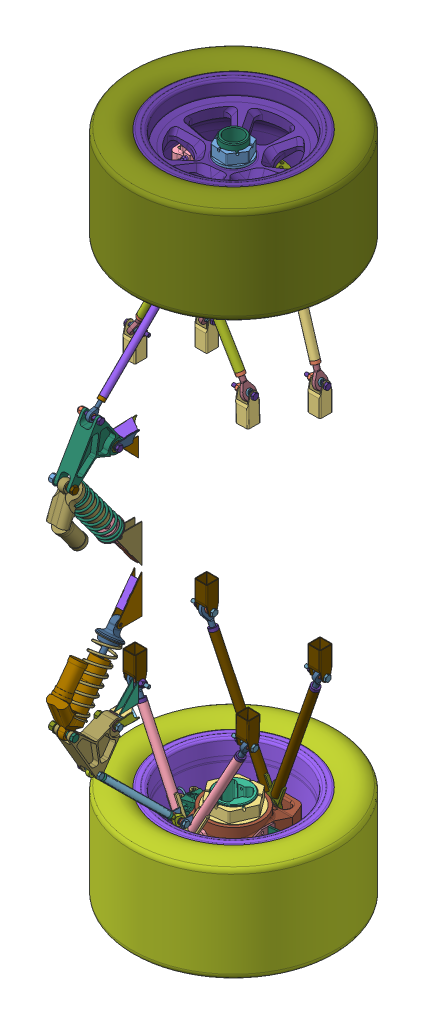
SolidWorks assembly UN-A1001-AA-Rear Unsprung Assembly, configuration Default. Lengths in mm. (continued)
Components (placement in the parent): (continued)
- MirrorWT-A0100-XG-Corner Assembly-2: MirrorWT-A0100-XG-Corner Assembly [Default] x (1 0 0) z (0 0 -1) size (411.48 213.6 411.53) (continued)
  - MirrorBR-A0000-AB-Rear Brake Assembly-1: MirrorBR-A0000-AB-Rear Brake Assembly [Default] at (-793.1174 596.9879 -198.9034) x (-0.602494 -0.000202 0.798123) z (0.798123 -0.000152 0.602494) size (251.55 172.72 251.55) (continued)
    - MirrorBR-20603-BA-Floating Bobbins-4: MirrorBR-20603-BA-Floating Bobbins [Default] at (-39.8696 25.9874 23.0188) x (-1 0 0) z (0 0 -1) size (15.88 8.92 15.88)
    - MirrorBR-20603-BA-Floating Bobbins-5: MirrorBR-20603-BA-Floating Bobbins [Default] at (0 25.9874 46.0375) x (-0.5 0 0.866025) z (-0.866025 0 -0.5) size (15.88 8.92 15.88)
    - MirrorBR-20603-BA-Floating Bobbins-6: MirrorBR-20603-BA-Floating Bobbins [Default] at (39.8696 25.9874 23.0188) x (0.5 0 0.866025) z (-0.866025 0 0.5) size (15.88 8.92 15.88)
    - MirrorWT-20104-AB-Rear Sensor Ring-1: MirrorWT-20104-AB-Rear Sensor Ring [Default] at (0 30.099 0) x (-0.882948 0 -0.469472) z (0 1 0) size (137 137 1.59)
    - Mirror91590A121_External Retaining Ring-1: Mirror91590A121_External Retaining Ring [91590A121] at (-39.8696 29.2354 -23.0188) x (0 1 0) z (0.857167 0 0.515038) size (0.64 14.63 13.25)
    - Mirror91590A121_External Retaining Ring-2: Mirror91590A121_External Retaining Ring [91590A121] at (-39.8696 29.2354 23.0188) x (0 1 0) z (0.87462 0 -0.48481) size (0.64 14.63 13.25)
    - Mirror91590A121_External Retaining Ring-3: Mirror91590A121_External Retaining Ring [91590A121] at (0 29.2354 46.0375) x (0 1 0) z (0.017452 0 -0.999848) size (0.64 14.63 13.25)
    - Mirror91590A121_External Retaining Ring-4: Mirror91590A121_External Retaining Ring [91590A121] at (39.8696 29.2354 23.0188) x (0 1 0) z (-0.857167 0 -0.515038) size (0.64 14.63 13.25)
    - Mirror91590A121_External Retaining Ring-5: Mirror91590A121_External Retaining Ring [91590A121] at (39.8696 29.2354 -23.0188) x (0 1 0) z (-0.87462 0 0.48481) size (0.64 14.63 13.25)
    - Mirror91590A121_External Retaining Ring-6: Mirror91590A121_External Retaining Ring [91590A121] at (0 29.2354 -46.0375) x (0 1 0) z (-0.017452 0 0.999848) size (0.64 14.63 13.25)
    - Mirror97447A110_Aluminum Blind Rivets with Aluminum Mandrel-1: Mirror97447A110_Aluminum Blind Rivets with Aluminum Mandrel [97447A110] at (9.6137 30.099 -51.8707) x (-0.302097 0 0.953277) z (0 -1 0) size (5.03 5.03 11.56)
    - Mirror97447A110_Aluminum Blind Rivets with Aluminum Mandrel-2: Mirror97447A110_Aluminum Blind Rivets with Aluminum Mandrel [97447A110] at (-40.1145 30.099 -34.261) x (0.674514 0 0.738262) z (0 -1 0) size (5.03 5.03 11.56)
    - Mirror97447A110_Aluminum Blind Rivets with Aluminum Mandrel-3: Mirror97447A110_Aluminum Blind Rivets with Aluminum Mandrel [97447A110] at (-49.7282 30.099 17.6097) x (0.976611 0 -0.215015) z (0 -1 0) size (5.03 5.03 11.56)
    - Mirror97447A110_Aluminum Blind Rivets with Aluminum Mandrel-4: Mirror97447A110_Aluminum Blind Rivets with Aluminum Mandrel [97447A110] at (-9.6137 30.099 51.8707) x (0.302097 0 -0.953277) z (0 -1 0) size (5.03 5.03 11.56)
    - Mirror97447A110_Aluminum Blind Rivets with Aluminum Mandrel-5: Mirror97447A110_Aluminum Blind Rivets with Aluminum Mandrel [97447A110] at (40.1145 30.099 34.261) x (-0.674514 0 -0.738262) z (0 -1 0) size (5.03 5.03 11.56)
    - Mirror97447A110_Aluminum Blind Rivets with Aluminum Mandrel-6: Mirror97447A110_Aluminum Blind Rivets with Aluminum Mandrel [97447A110] at (49.7282 30.099 -17.6097) x (-0.976611 0 0.215015) z (0 -1 0) size (5.03 5.03 11.56)
  - MirrorFS-Jet Nut, M8x1.25 (MJET-M8X1.25)-1: MirrorFS-Jet Nut, M8x1.25 (MJET-M8X1.25) [Default] at (-816.1783 561.0546 -293.5333) x (-0.906747 0.01433 0.421432) z (0.000308 -0.9994 0.034645) size (13.6 13.6 7)
  - Mirror91290A442_Alloy Steel Socket Head Screw-2: Mirror91290A442_Alloy Steel Socket Head Screw [91290A442] at (-771.7287 556.8303 -293.7791) x (-0.549228 0.028783 0.835176) z (-0.000308 0.9994 -0.034645) size (13 13 48.09)
  - MirrorFS-Jet Nut, M8x1.25 (MJET-M8X1.25)-2: MirrorFS-Jet Nut, M8x1.25 (MJET-M8X1.25) [Default] at (-771.73 561.0547 -293.9256) x (0.139109 0.034351 0.989681) z (0.000308 -0.9994 0.034645) size (13.6 13.6 7)
  - MirrorWT-10105-AA-Drive Pin-2: MirrorWT-10105-AA-Drive Pin [Default] at (-769.0177 596.9959 -230.8283) x (0.992582 0.000031 -0.121576) z (0.121576 -0.000251 0.992582) size (12.67 23.01 11.95)
  - MirrorWT-10105-AA-Drive Pin-3: MirrorWT-10105-AA-Drive Pin [Default] at (-761.1925 596.9818 -174.8036) x (0.121576 -0.000251 0.992582) z (-0.992582 -0.000031 0.121576) size (12.67 23.01 11.95)
  - MirrorWT-10105-AA-Drive Pin-4: MirrorWT-10105-AA-Drive Pin [Default] at (-817.2172 596.9798 -166.9785) x (-0.992582 -0.000031 0.121576) z (-0.121576 0.000251 -0.992582) size (12.67 23.01 11.95)
  - MirrorWT-AA-#####-Rear Toe Backing Plate-1: MirrorWT-AA-#####-Rear Toe Backing Plate [Default] at (-737.6079 537.8924 -199.4082) x (0.999961 0.000002 -0.008824) z (0.008824 -0.000253 0.999961) size (3.17 25.4 50.8)
  - MirrorWT-AA-#####-Rear Toe Top Clevis-1: MirrorWT-AA-#####-Rear Toe Top Clevis [Default] at (-737.7085 541.0703 -210.8115) x (0.999961 0.000002 -0.008824) z (0.008824 -0.000253 0.999961) size (31.75 27.83 3.17)
  - MirrorWT-AA-#####-Rear Toe Bottom Clevis-1: MirrorWT-AA-#####-Rear Toe Bottom Clevis [Default] at (-737.4815 537.8888 -185.0832) x (0.999961 0.000002 -0.008824) z (0.008824 -0.000253 0.999961) size (31.75 27.12 3.17)
- MirrorSP-A0200-AH-Rear Axle Assembly-3: MirrorSP-A0200-AH-Rear Axle Assembly [Default] x (1 0 0) z (0 0 -1) size (274.88 563.57 484.64)
  - MirrorSP-AA-Rear Lower A-Arm^SP-A0200-AH-Rear Axle Assembly-1: MirrorSP-AA-Rear Lower A-Arm^SP-A0200-AH-Rear Axle Assembly [Default] at (0 -0.399 -0.6588) x (1 0 0) z (0 -0.002866 0.999996) size (222.76 290.57 36.42)
    - MirrorSP-Lower Apex Rear-1: MirrorSP-Lower Apex Rear [Default] at (-792.4265 549.6462 -121.5417) x (-0.932505 -0.360479 -0.022123) z (0 0.061256 -0.998122) size (54.94 63.8 9.53)
    - MirrorMirrorFS-MALE ROD END UNF-3A, 0.3125x24-0.25D (XAM-4)14-1: MirrorMirrorFS-MALE ROD END UNF-3A, 0.3125x24-0.25D (XAM-4)14 [Default] at (-906.7265 255.0788 -139.6197) x (0.932505 -0.360479 -0.022123) z (0.361157 0.930754 0.057121)
    - MirrorMirrorFS-MALE ROD END UNF-3A, 0.3125x24-0.25D (XAM-4)15-1: MirrorMirrorFS-MALE ROD END UNF-3A, 0.3125x24-0.25D (XAM-4)15 [Default] at (-678.1265 255.0788 -139.6197) x (0.932505 0.360479 0.022123) z (-0.361157 0.930754 0.057121)
    - MirrorSP-10003-AB-Threaded Insert-1: MirrorSP-10003-AB-Threaded Insert [A-Arm] at (-890.6731 296.4508 -137.0806) x (0.932505 -0.360479 -0.022123) z (0.361157 0.930754 0.057121) size (15.88 15.88 15.88)
    - MirrorSP-10003-AB-Threaded Insert-2: MirrorSP-10003-AB-Threaded Insert [A-Arm] at (-694.18 296.4508 -137.0806) x (0.932505 0.360479 0.022123) z (-0.361157 0.930754 0.057121) size (15.88 15.88 15.88)
    - MirrorSP-Rear Lower A-Arm Tube-1: MirrorSP-Rear Lower A-Arm Tube [Default] at (-838.6322 430.5677 -128.8497) x (-0.361157 -0.930754 -0.057121) z (0 0.061256 -0.998122) size (257.84 15.88 15.88)
    - MirrorSP-Rear Lower A-Arm Tube-2: MirrorSP-Rear Lower A-Arm Tube [Default] at (-746.2209 430.5677 -128.8497) x (0.361157 -0.930754 -0.057121) z (0 -0.061256 0.998122) size (257.84 15.88 15.88)
    - MirrorFS-HIGH MISALIGN SPHERICAL BEARING, 0.375-0.906D (3072-6G)2-1: MirrorFS-HIGH MISALIGN SPHERICAL BEARING, 0.375-0.906D (3072-6G)2 [Default] at (-792.4265 549.6462 -121.5417) x (-0.932505 0.360479 0.022123) z (0.361157 0.930754 0.057121) size (26.46 21.71 26.13)
      - MirrorRace^FS-HIGH MISALIGN SPHERICAL BEARING, 0.375-0.906D (3072-6G)-1: MirrorRace^FS-HIGH MISALIGN SPHERICAL BEARING, 0.375-0.906D (3072-6G) [Default] at origin size (23.01 8.76 23.01) (virtual)
      - MirrorBall^FS-HIGH MISALIGN SPHERICAL BEARING, 0.375-0.906D (3072-6G)-1: MirrorBall^FS-HIGH MISALIGN SPHERICAL BEARING, 0.375-0.906D (3072-6G) [Default] x (0.359576 -0.008176 -0.93308) z (0.932238 0.046516 0.358844) size (19.84 20.65 19.84) (virtual)
  - MirrorSP-AA-Rear Upper A-Arm^SP-A0200-AH-Rear Axle Assembly-1: MirrorSP-AA-Rear Upper A-Arm^SP-A0200-AH-Rear Axle Assembly [Default] at (-38.1 -1.9308 -1.9372) x (1 0 0) z (0 -0.00685 0.999977) size (216 215.55 29.43)
    - MirrorSP-Upper Apex Rear-1: MirrorSP-Upper Apex Rear [Default] at (-755.8405 523.8827 -293.8505) x (0.884705 -0.465567 0.023329) z (0 0.050046 0.998747) size (76.45 83.12 9.53)
    - MirrorMirrorFS-MALE ROD END UNF-3A, 0.3125x24-0.25D (XAM-4)16-1: MirrorMirrorFS-MALE ROD END UNF-3A, 0.3125x24-0.25D (XAM-4)16 [Default] at (-870.1405 307.2255 -282.9942) x (0.884705 -0.465567 0.023329) z (0.466151 0.883596 -0.044276)
    - MirrorMirrorFS-MALE ROD END UNF-3A, 0.3125x24-0.25D (XAM-4)17-1: MirrorMirrorFS-MALE ROD END UNF-3A, 0.3125x24-0.25D (XAM-4)17 [Default] at (-641.5405 307.2255 -282.9942) x (0.884705 0.465567 -0.023329) z (-0.466151 0.883596 -0.044276)
    - MirrorSP-10003-AB-Threaded Insert-1: MirrorSP-10003-AB-Threaded Insert [A-Arm] at (-849.4201 346.5014 -284.9623) x (0.884705 -0.465567 0.023329) z (0.466151 0.883596 -0.044276) size (15.88 15.88 15.88)
    - MirrorSP-10003-AB-Threaded Insert-2: MirrorSP-10003-AB-Threaded Insert [A-Arm] at (-662.261 346.5014 -284.9623) x (0.884705 0.465567 -0.023329) z (-0.466151 0.883596 -0.044276) size (15.88 15.88 15.88)
    - MirrorSP-Rear Upper A-Arm Tube-1: MirrorSP-Rear Upper A-Arm Tube [Default] at (-812.9905 415.5541 -288.4224) x (0.466151 0.883596 -0.044276) z (-0.884705 0.465567 -0.023329) size (186.28 15.88 15.88)
    - MirrorSP-Rear Upper A-Arm Tube-2: MirrorSP-Rear Upper A-Arm Tube [Default] at (-698.6905 415.5541 -288.4224) x (-0.466151 0.883596 -0.044276) z (-0.884705 -0.465567 0.023329) size (186.28 15.88 15.88)
    - MirrorFS-HIGH MISALIGN SPHERICAL BEARING, 0.375-0.906D (3072-6G)3-1: MirrorFS-HIGH MISALIGN SPHERICAL BEARING, 0.375-0.906D (3072-6G)3 [Default] at (-755.8405 523.8827 -293.8505) x (0.884705 -0.465567 0.023329) z (0.466151 0.883596 -0.044276) size (26.46 21.71 26.13)
      - MirrorRace^FS-HIGH MISALIGN SPHERICAL BEARING, 0.375-0.906D (3072-6G)-1: MirrorRace^FS-HIGH MISALIGN SPHERICAL BEARING, 0.375-0.906D (3072-6G) [Default] at origin size (23.01 8.76 23.01) (virtual)
      - MirrorBall^FS-HIGH MISALIGN SPHERICAL BEARING, 0.375-0.906D (3072-6G)-1: MirrorBall^FS-HIGH MISALIGN SPHERICAL BEARING, 0.375-0.906D (3072-6G) [Default] x (0.359576 -0.008176 -0.93308) z (0.932238 0.046516 0.358844) size (19.84 20.65 19.84) (virtual)
  - MirrorAssem8^SP-A0200-AH-Rear Axle Assembly-1: MirrorAssem8^SP-A0200-AH-Rear Axle Assembly [Default] at (-1592.9214 814.7933 -712.2762) x (-0.999891 -0.01037 -0.010464) z (-0.012143 0.982316 0.186836) size (17.98 166.51 230.13)
    - MirrorPart2^Assem8_SP-A0200-AH-Rear Axle Assembly-1: MirrorPart2^Assem8_SP-A0200-AH-Rear Axle Assembly [Default] at origin size (15.39 113.92 157.78) (virtual)
    - MirrorSP-10003-AC-Threaded Insert-1: MirrorSP-10003-AC-Threaded Insert [AM-4 Rod End Thread] at (-799.064 427.6015 -294.0449) x (-0.999891 -0.008342 -0.012143) z (0.014733 -0.566176 -0.824153) size (12.7 12.7 15.88)
    - MirrorSP-10003-AC-Threaded Insert-2: MirrorSP-10003-AC-Threaded Insert [AM-4 Rod End Thread] at (-796.6527 334.9355 -428.9338) x (-0.999891 -0.008342 -0.012143) z (-0.014733 0.566176 0.824153) size (12.7 12.7 15.88)
    - MirrorFS-MALE ROD END UNF-3A, 0.25x28-0.25D (AM-4)2-1: MirrorFS-MALE ROD END UNF-3A, 0.25x28-0.25D (AM-4)2 [Default] at (-796.0446 311.5665 -462.9507) x (0 -0.824242 0.566238) z (0.014733 -0.566176 -0.824153) size (19.32 14.06 49.44)
      - MirrorBody^FS-MALE ROD END UNF-3A, 0.25x28-0.25D (AM-4)-1: MirrorBody^FS-MALE ROD END UNF-3A, 0.25x28-0.25D (AM-4) [Default] at origin size (19.32 7.2 49.44) (virtual)
      - MirrorBall^FS-MALE ROD END UNF-3A, 0.25x28-0.25D (AM-4)-1: MirrorBall^FS-MALE ROD END UNF-3A, 0.25x28-0.25D (AM-4) [Default] x (0.09633 0.218783 -0.971007) z (0.984027 -0.167661 0.059845) size (12.7 9.53 12.7) (virtual)
    - MirrorFS-MALE ROD END UNF-3A, 0.25x28-0.25D (AM-4)3-1: MirrorFS-MALE ROD END UNF-3A, 0.25x28-0.25D (AM-4)3 [Default] at (-799.6721 450.9704 -260.028) x (0 -0.824242 0.566238) z (-0.014733 0.566176 0.824153) size (19.32 14.06 49.44)
      - MirrorBody^FS-MALE ROD END UNF-3A, 0.25x28-0.25D (AM-4)-1: MirrorBody^FS-MALE ROD END UNF-3A, 0.25x28-0.25D (AM-4) [Default] at origin size (19.32 7.2 49.44) (virtual)
      - MirrorBall^FS-MALE ROD END UNF-3A, 0.25x28-0.25D (AM-4)-1: MirrorBall^FS-MALE ROD END UNF-3A, 0.25x28-0.25D (AM-4) [Default] x (0.09633 0.218783 -0.971007) z (0.984027 -0.167661 0.059845) size (12.7 9.53 12.7) (virtual)
  - MirrorSP-A0105-AC-Ohlin TTX25 MKII, 200mm1-1: MirrorSP-A0105-AC-Ohlin TTX25 MKII, 200mm1 [Default] at (-793.9406 216.4917 -537.8809) x (-1 0 0) z (0 -0.803503 0.5953) size (48.39 85.02 197.6)
    - MirrorShock Body^SP-A0105-AC-Ohlin TTX25 MKII, 200mm-1: MirrorShock Body^SP-A0105-AC-Ohlin TTX25 MKII, 200mm [Default] at origin size (40.76 80 131.7) (virtual)
    - MirrorHead^SP-A0105-AC-Ohlin TTX25 MKII, 200mm-1: MirrorHead^SP-A0105-AC-Ohlin TTX25 MKII, 200mm [Default] at (0 0 174.6) size (46 46 119) (virtual)
    - MirrorBall^SP-A0105-AC-Ohlin TTX25 MKII, 200mm-1: MirrorBall^SP-A0105-AC-Ohlin TTX25 MKII, 200mm [Default] at (0 0 174.6) x (-0.011681 0.107343 -0.994153) z (-0.993776 -0.111394 -0.000351) size (15 15 8) (virtual)
    - MirrorBall^SP-A0105-AC-Ohlin TTX25 MKII, 200mm-2: MirrorBall^SP-A0105-AC-Ohlin TTX25 MKII, 200mm [Default] x (0.079523 -0.862756 0.499328) z (-0.965926 0.057074 0.252448) size (15 15 8) (virtual)
    - MirrorSP-#####-AB-Spring-1: MirrorSP-#####-AB-Spring [Default] at (0 0 151.1) size (48.39 49.05 127.97)
  - MirrorFS-BALL BEARING, 0.25ID-0.75OD (60355K702)-1: MirrorFS-BALL BEARING, 0.25ID-0.75OD (60355K702) [Default] at (-784.8125 243.84 -446.6415) x (0 -0.287121 -0.957894) z (1 0 0) size (19.05 19.05 7.14)
  - MirrorFS-BALL BEARING, 0.25ID-0.75OD (60355K702)-2: MirrorFS-BALL BEARING, 0.25ID-0.75OD (60355K702) [Default] at (-803.0688 243.84 -446.6415) x (0 0.287121 0.957894) z (-1 0 0) size (19.05 19.05 7.14)
  - MirrorFS-CADMIUM PLATED C3 HEX, 0.25x28-1.65-0.469 (AN4-13A)-1: MirrorFS-CADMIUM PLATED C3 HEX, 0.25x28-1.65-0.469 (AN4-13A) [Default] at (-796.8362 310.0391 -484.3789) x (-1 0 0) z (0 -0.868755 0.495242) size (46.28 12.9 11.18)
  - MirrorFS-ZINC YELLOW CHROMATE C10.9 HX, M8x1.25-40-22 (95327A569)-1: MirrorFS-ZINC YELLOW CHROMATE C10.9 HX, M8x1.25-40-22 (95327A569) [Default] at (-795.4156 216.4917 -537.8809) x (-1 0 0) z (0 0.287121 0.957894) size (45.3 15.01 13)
  - MirrorFS-NYLOC FLHX C8, M8x1.25-11.1 (92461A400)-1: MirrorFS-NYLOC FLHX C8, M8x1.25-11.1 (92461A400) [Default] at (-820.9156 216.4917 -537.8809) x (0 0.868058 0.496463) z (1 0 0) size (17.9 17.9 11.1)
  - MirrorFS-NYLOC G8 HX, 0.25x28-0.3125 (90630A145)-1: MirrorFS-NYLOC G8 HX, 0.25x28-0.3125 (90630A145) [Default] at (-809.8156 310.0391 -484.3789) x (0 0.868058 0.496463) z (0 -0.496463 0.868058) size (11.11 7.94 12.83)
  - MirrorSP-C30066-AA-A-Arm Tab Box-1: MirrorSP-C30066-AA-A-Arm Tab Box [Default] at (-680.9758 289.7175 -282.8202) x (-0.029021 0.999579 0) z (0 0 -1) size (60.32 25.4 25.4)
  - MirrorSP-C30066-AA-A-Arm Tab Box-2: MirrorSP-C30066-AA-A-Arm Tab Box [Default] at (-908.2405 289.7636 -282.8202) x (0 1 0) z (0 0 -1) size (60.32 25.4 25.4)
  - MirrorSP-C30066-AA-A-Arm Tab Box-3: MirrorSP-C30066-AA-A-Arm Tab Box [Default] at (-678.1265 237.6164 -139.5469) x (0 1 0) z (0 0 1) size (60.32 25.4 25.4)
  - MirrorSP-C30066-AA-A-Arm Tab Box-4: MirrorSP-C30066-AA-A-Arm Tab Box [Default] at (-906.7265 237.6164 -139.5469) x (0 1 0) z (0 0 1) size (60.32 25.4 25.4)
  - MirrorMirrorSP-30063-AB-Pushrod Tab-1: MirrorMirrorSP-30063-AB-Pushrod Tab [Default] at (-782.0343 483.2134 -293.6084) x (1 0 0) z (0 -0.043203 -0.999066) size (1.59 15.88 23.81)
  - MirrorMirrorSP-30063-AB-Pushrod Tab-2: MirrorMirrorSP-30063-AB-Pushrod Tab [Default] at (-805.8468 483.2134 -293.6084) x (-1 0 0) z (0 -0.043203 -0.999066) size (1.59 15.88 23.81)
  - MirrorFS-NYLOC FLHX C8, M8x1.25-11.1 (92461A400)-2: MirrorFS-NYLOC FLHX C8, M8x1.25-11.1 (92461A400) [Default] at (-820.9156 243.84 -446.6415) x (0 0 1) z (1 0 0) size (17.9 17.9 11.1)
  - MirrorFS-CADMIUM PLATED C3 HEX, 0.25x28-1.65-0.469 (AN4-13A)-2: MirrorFS-CADMIUM PLATED C3 HEX, 0.25x28-1.65-0.469 (AN4-13A) [Default] at (-796.8362 243.84 -446.6415) x (-1 0 0) z (0 -0.287121 -0.957894) size (46.28 12.9 11.18)
  - MirrorFS-CADMIUM PLATED C3 HEX, 0.25x28-1.65-0.469 (AN4-13A)-3: MirrorFS-CADMIUM PLATED C3 HEX, 0.25x28-1.65-0.469 (AN4-13A) [Default] at (-687.5506 306.9965 -282.8202) x (-0.999579 -0.029021 0) z (0 0 -1) size (46.28 12.9 11.18)
  - MirrorFS-CADMIUM PLATED C3 HEX, 0.25x28-1.65-0.469 (AN4-13A)-4: MirrorFS-CADMIUM PLATED C3 HEX, 0.25x28-1.65-0.469 (AN4-13A) [Default] at (-902.1699 307.2261 -282.8202) size (46.28 12.9 11.18)
  - MirrorFS-CADMIUM PLATED C3 HEX, 0.25x28-1.65-0.469 (AN4-13A)-5: MirrorFS-CADMIUM PLATED C3 HEX, 0.25x28-1.65-0.469 (AN4-13A) [Default] at (-912.7971 255.0789 -139.5469) x (-1 0 0) z (0 0 -1) size (46.28 12.9 11.18)
  - MirrorFS-CADMIUM PLATED C3 HEX, 0.25x28-1.65-0.469 (AN4-13A)-6: MirrorFS-CADMIUM PLATED C3 HEX, 0.25x28-1.65-0.469 (AN4-13A) [Default] at (-684.1971 255.0789 -139.5469) x (-1 0 0) z (0 0 -1) size (46.28 12.9 11.18)
  - MirrorFS-CADMIUM PLATED C3 HEX, 0.25x28-1.65-0.469 (AN4-13A)-7: MirrorFS-CADMIUM PLATED C3 HEX, 0.25x28-1.65-0.469 (AN4-13A) [Default] at (-799.2174 482.5275 -309.4686) x (-1 0 0) z (0 0.609051 0.793131) size (46.28 12.9 11.18)
  - MirrorFS-NYLOC G8 HX, 0.25x28-0.3125 (90630A145)-2: MirrorFS-NYLOC G8 HX, 0.25x28-0.3125 (90630A145) [Default] at (-807.4343 482.5275 -309.4686) x (0 -0.043203 -0.999066) z (0 0.999066 -0.043203) size (11.11 7.94 12.83)
  - MirrorFS-NYLOC G8 HX, 0.25x28-0.3125 (90630A145)-3: MirrorFS-NYLOC G8 HX, 0.25x28-0.3125 (90630A145) [Default] at (-694.1772 306.8041 -282.8202) x (-0.029021 0.999579 0) z (0 0 1) size (11.11 7.94 12.83)
  - MirrorFS-NYLOC G8 HX, 0.25x28-0.3125 (90630A145)-4: MirrorFS-NYLOC G8 HX, 0.25x28-0.3125 (90630A145) [Default] at (-895.5405 307.2261 -282.8202) x (0 1 0) z (0 0 -1) size (11.11 7.94 12.83)
  - MirrorFS-NYLOC G8 HX, 0.25x28-0.3125 (90630A145)-5: MirrorFS-NYLOC G8 HX, 0.25x28-0.3125 (90630A145) [Default] at (-919.4265 255.0789 -139.5469) x (0 1 0) z (0 0 1) size (11.11 7.94 12.83)
  - MirrorFS-NYLOC G8 HX, 0.25x28-0.3125 (90630A145)-6: MirrorFS-NYLOC G8 HX, 0.25x28-0.3125 (90630A145) [Default] at (-690.8265 255.0789 -139.5469) x (0 -1 0) z (0 0 -1) size (11.11 7.94 12.83)
  - MirrorFS-ROD END RETAINING WASHER, 0.25-0.245 (NO PN)-1: MirrorFS-ROD END RETAINING WASHER, 0.25-0.245 (NO PN) [Default] at (-781.9073 482.5275 -309.4686) x (0 1 0) z (1 0 0) size (12.7 12.7 6.22)
  - MirrorFS-ROD END RETAINING WASHER, 0.25-0.245 (NO PN)-2: MirrorFS-ROD END RETAINING WASHER, 0.25-0.245 (NO PN) [Default] at (-805.9738 482.5275 -309.4686) x (0 0.978954 -0.204082) z (-1 0 0) size (12.7 12.7 6.22)
  - MirrorSP-A0200-Rear Inner Rocker Gusset-1: MirrorSP-A0200-Rear Inner Rocker Gusset [Default] at (-793.9406 234.6955 -425.4808) x (1 0 0) z (0 -0.052336 0.99863) size (26.99 1.59 48.67)
  - MirrorSP-A0200-Rear Long Rocker Tab-1: MirrorSP-A0200-Rear Long Rocker Tab [Rear] at (-807.4344 243.84 -446.6415) x (1 0 0) z (0 0.00621 -0.999981) size (1.59 19.05 73.11)
  - MirrorSP-A0200-Rear Outer Rocker Gusset-1: MirrorSP-A0200-Rear Outer Rocker Gusset [Default] at (-793.9406 251.3902 -418.9606) x (1 0 0) z (0 0.039929 0.999203) size (26.99 1.59 43.52)
  - MirrorSP-A0200-Rear Rocker Gusset Support-1: MirrorSP-A0200-Rear Rocker Gusset Support [Default] at (-800.2906 228.5949 -403.7833) x (0 0 -1) z (0 -1 0) size (38.05 1.59 40.09)
  - MirrorSP-A0200-Rear Short Rocker Tab-1: MirrorSP-A0200-Rear Short Rocker Tab [Rear] at (-780.4469 243.8408 -446.6212) x (1 0 0) z (0 0.00621 -0.999981) size (1.59 17.17 50.59)
  - MirrorSP-A0200-Rear Rocker Gusset Support-2: MirrorSP-A0200-Rear Rocker Gusset Support [Default] at (-789.8131 228.5949 -403.7833) x (0 0 -1) z (0 -1 0) size (38.05 1.59 40.09)
  - MirrorSP-A0200-Rear Shock Gusset-1: MirrorSP-A0200-Rear Shock Gusset [Default] at (-793.9406 34.3591 -413.4634) x (1 0 0) z (0 -0.809017 0.587785) size (14.29 1.59 50.8)
  - MirrorSP-A0200-Rear Shock Tab-1: MirrorSP-A0200-Rear Shock Tab [Rear] at (-786.7969 76.2 -433.9415) x (-1 0 0) z (0 0.809017 -0.587785) size (1.59 45.95 88.76)
  - MirrorSP-A0200-Rear Shock Tab-2: MirrorSP-A0200-Rear Shock Tab [Front] at (-801.0844 76.2 -433.9415) x (-1 0 0) z (0 0.809017 -0.587785) size (1.59 45.95 88.76)
  - MirrorFS-MALE ROD END UNJF-3A, 0.375x24-0.25D (HXAM-4T)4-1: MirrorFS-MALE ROD END UNJF-3A, 0.375x24-0.25D (HXAM-4T)4 [Default] at (-679.6405 307.2261 -282.8202) x (0 0.043203 0.999066) z (0.466151 -0.883879 0.038222) size (26.22 15.06 62.54)
    - MirrorBody^FS-MALE ROD END UNJF-3A, 0.375x24-0.25D (HXAM-4T)-1: MirrorBody^FS-MALE ROD END UNJF-3A, 0.375x24-0.25D (HXAM-4T) [no_threads] at origin size (26.22 9.62 62.54)
    - MirrorBall^FS-MALE ROD END UNJF-3A, 0.375x24-0.25D (HXAM-4T)-1: MirrorBall^FS-MALE ROD END UNJF-3A, 0.375x24-0.25D (HXAM-4T) [Default] at origin size (15.06 15.06 15.06)
  - MirrorFS-MALE ROD END UNJF-3A, 0.375x24-0.25D (HXAM-4T)5-1: MirrorFS-MALE ROD END UNJF-3A, 0.375x24-0.25D (HXAM-4T)5 [Default] at (-908.2405 307.2261 -282.8202) x (0 -0.043203 -0.999066) z (-0.466151 -0.883879 0.038222) size (26.22 15.06 62.54)
    - MirrorBody^FS-MALE ROD END UNJF-3A, 0.375x24-0.25D (HXAM-4T)-1: MirrorBody^FS-MALE ROD END UNJF-3A, 0.375x24-0.25D (HXAM-4T) [no_threads] at origin size (26.22 9.62 62.54)
    - MirrorBall^FS-MALE ROD END UNJF-3A, 0.375x24-0.25D (HXAM-4T)-1: MirrorBall^FS-MALE ROD END UNJF-3A, 0.375x24-0.25D (HXAM-4T) [Default] at origin size (15.06 15.06 15.06)
  - MirrorFS-MALE ROD END UNJF-3A, 0.375x24-0.25D (HXAM-4T)6-1: MirrorFS-MALE ROD END UNJF-3A, 0.375x24-0.25D (HXAM-4T)6 [Default] at (-906.7265 255.0789 -139.5469) x (0 0.064116 -0.997942) z (-0.361157 -0.930586 -0.059789) size (26.22 15.06 62.54)
    - MirrorBody^FS-MALE ROD END UNJF-3A, 0.375x24-0.25D (HXAM-4T)-1: MirrorBody^FS-MALE ROD END UNJF-3A, 0.375x24-0.25D (HXAM-4T) [no_threads] at origin size (26.22 9.62 62.54)
    - MirrorBall^FS-MALE ROD END UNJF-3A, 0.375x24-0.25D (HXAM-4T)-1: MirrorBall^FS-MALE ROD END UNJF-3A, 0.375x24-0.25D (HXAM-4T) [Default] at origin size (15.06 15.06 15.06)
  - MirrorFS-MALE ROD END UNJF-3A, 0.375x24-0.25D (HXAM-4T)7-1: MirrorFS-MALE ROD END UNJF-3A, 0.375x24-0.25D (HXAM-4T)7 [Default] at (-678.1265 255.0789 -139.5469) x (0 -0.064116 0.997942) z (0.361157 -0.930586 -0.059789) size (26.22 15.06 62.54)
    - MirrorBody^FS-MALE ROD END UNJF-3A, 0.375x24-0.25D (HXAM-4T)-1: MirrorBody^FS-MALE ROD END UNJF-3A, 0.375x24-0.25D (HXAM-4T) [no_threads] at origin size (26.22 9.62 62.54)
    - MirrorBall^FS-MALE ROD END UNJF-3A, 0.375x24-0.25D (HXAM-4T)-1: MirrorBall^FS-MALE ROD END UNJF-3A, 0.375x24-0.25D (HXAM-4T) [Default] at origin size (15.06 15.06 15.06)
  - MirrorSP-B0100-Rear Rocker-1: MirrorSP-B0100-Rear Rocker [Default] at (14.7593 458.8134 310.4211) x (0.993764 -0.111506 0.000215) z (0.085107 0.759728 0.644647) size (43.51 92.41 122.03)
Mates (geometry in assembly coordinates):
- Coincident1: coincident: point of ?
- Coincident2: coincident: line of SP-A0200-AH-Rear Axle Assembly-1 through (307.2261 -793.9405 0) axis (0 0 1)
- Coincident3: coincident: line of SP-A0200-AH-Rear Axle Assembly-1 through (0 792.4265 0) axis (0 0 -1)
- Parallel1: parallel: line of SP-A0200-AH-Rear Axle Assembly-1 through (307.2261 -793.9405 0) axis (0 0 1)
- Parallel2: parallel: line of SP-A0200-AH-Rear Axle Assembly-1 through (0 792.4265 0) axis (0 0 -1)
- Coincident5: coincident: point of SP-A0200-AH-Rear Axle Assembly-1; point of WT-A0100-XG-Corner Assembly-1
- Coincident6: coincident aligned: line of SP-A0200-AH-Rear Axle Assembly-1 through (0 792.4265 0) axis (0 0 -1); line of WT-A0100-XG-Corner Assembly-1 through (0 792.4265 0) axis (0 0 -1)
- Coincident7: coincident aligned: line of SP-A0200-AH-Rear Axle Assembly-1 through (307.2261 -793.9405 0) axis (0 0 1); line of WT-A0100-XG-Corner Assembly-1 through (307.2261 -793.9405 0) axis (0 0 1)
